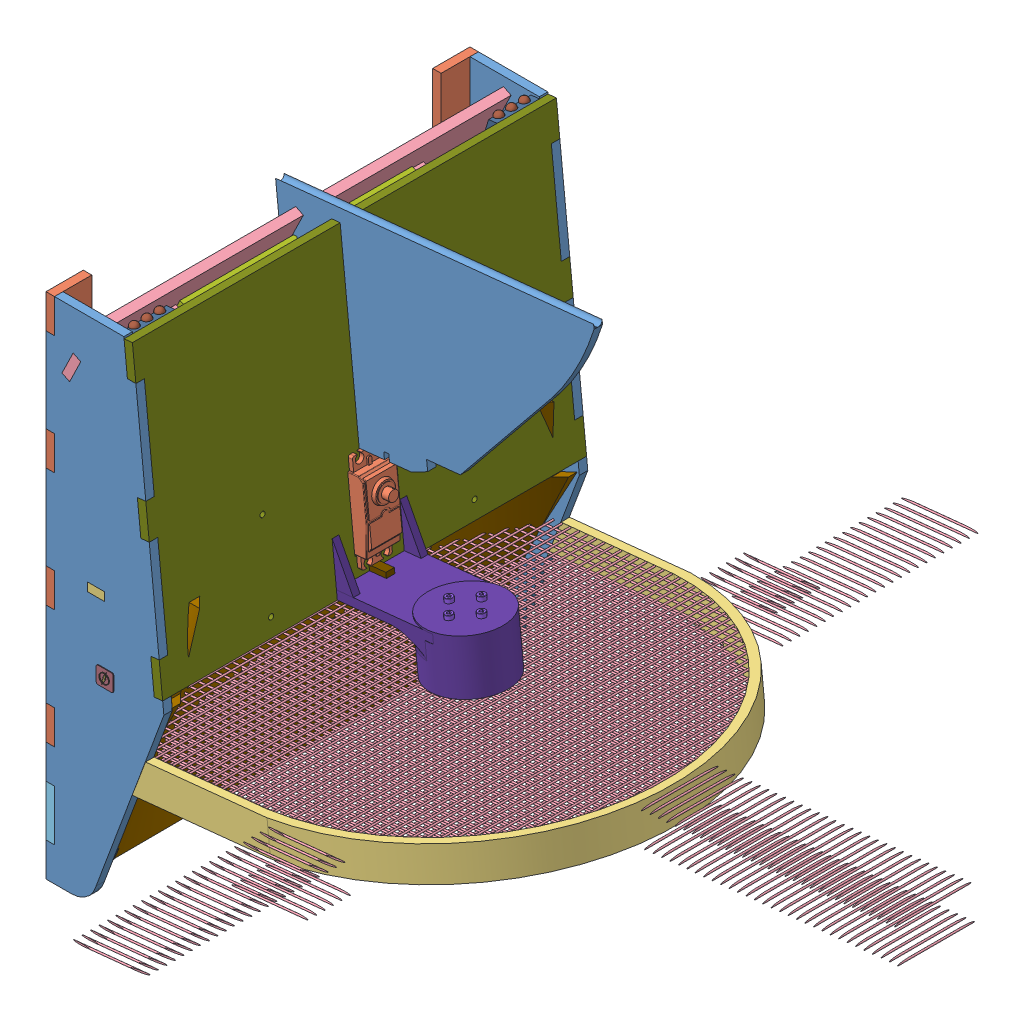
SolidWorks assembly AssStructSimu, configuration Défaut. Lengths in mm.
Overall size (253.25 324.59 251.6).
1750 component instances, 226 part files, 11 mates.
Components (placement in the parent):
- AssBase-1: AssBase [Défaut] at (36.5482 -71.0398 34.0612) size (86.08 302.3 251.6)
  - AssD-1: AssD [Défaut] at (39.0992 31.0201 8.5) size (69.5 300 22)
    - P1-1: P1 [Défaut] at (-95.5819 194.6656 377.5) size (69.5 300 5)
    - P5-1: P5 [Défaut] at (-100.5819 -35.3344 360.5) x (0 1 0) z (1 0 0) size (230 22 5)
  - AssG-1: AssG [Défaut] at (39.0992 31.0201 -236.5) size (69.5 300 22)
    - P1-1: P1 [Défaut] at (-95.5819 194.6656 377.5) size (69.5 300 5)
    - P5-1: P5 [Défaut] at (-95.5819 -35.3344 399.5) x (0 1 0) z (-1 0 0) size (230 22 5)
  - P7-1: P7 [Défaut] at (-1.4828 89.6857 370.5) x (0 0 -1) z (0 -1 0) size (250 54.5 5)
  - P4-1: P4 [Défaut] at (-63.2363 165.9323 386) x (0 0 -1) z (0.898794 -0.438371 0) size (250 60.5 66.27)
  - P3-1: P3 [Défaut] at (-56.4828 -74.3143 146) x (0 0 1) z (-1 0 0) size (250 70 5)
  - P4b-1: P4b [Défaut] at (-58.7423 163.7404 190) x (0 0 1) z (0.438371 0.898794 0) size (152 56 2)
  - battery-1: battery [Défaut] at (-39.0156 204.1861 197.5) x (0 0 1) z (0.898794 -0.438371 0) size (137 43 30)
  - socket head cap screw 4762_din-1: socket head cap screw 4762_din [EN ISO 4762 M3 x 10 - 10N] at (-27.7008 145.2627 193) x (0.438371 0.898794 0) z (0 0 -1) size (13 5.5 5.5)
  - socket head cap screw 4762_din-2: socket head cap screw 4762_din [EN ISO 4762 M3 x 10 - 10N] at (-27.7008 145.2627 339) x (0.438371 0.898794 0) z (-0.791285 0.385936 -0.474259) size (13 5.5 5.5)
  - socket head cap screw 4762_din-3: socket head cap screw 4762_din [EN ISO 4762 M3 x 10 - 10N] at (-42.0815 152.2766 339) x (0.438371 0.898794 0) z (-0.001489 0.000726 -0.999999) size (13 5.5 5.5)
  - socket head cap screw 4762_din-4: socket head cap screw 4762_din [EN ISO 4762 M3 x 10 - 10N] at (-42.0815 152.2766 193) x (0.438371 0.898794 0) z (-0.031331 0.015281 -0.999392) size (13 5.5 5.5)
  - P11-1: P11 [Défaut] at (-57.5734 -73.9703 146.7843) x (0.005072 0 0.999987) z (0.006197 0.999981 -0.000031) size (240 65 164)
  - AssPhare-1: AssPhare [Défaut] at (-52.8518 -67.6977 411) x (0 1 0) z (0 0 -1) size (40.8 8 27.06)
    - piece_led-1: piece_led [Défaut] at (-6.6166 -3.631 25) size (7 8 25)
    - LED 5mm-1: LED 5mm [Valor predeterminado] at (-0.1166 0.369 30) x (0 0 1) z (-1 0 0) size (5.5 6 35.8)
    - LED 5mm-2: LED 5mm [Valor predeterminado] at (-0.1166 0.369 37.5) x (0 0 1) z (-1 0 0) size (5.5 6 35.8)
    - LED 5mm-3: LED 5mm [Valor predeterminado] at (-0.1166 0.369 45) x (0 0 1) z (-1 0 0) size (5.5 6 35.8)
  - AssPhare-2: AssPhare [Défaut] at (-52.8518 -67.6977 196) x (0 1 0) z (0 0 -1) size (40.8 8 27.06)
    - piece_led-1: piece_led [Défaut] at (-6.6166 -3.631 25) size (7 8 25)
    - LED 5mm-1: LED 5mm [Valor predeterminado] at (-0.1166 0.369 30) x (0 0 1) z (-1 0 0) size (5.5 6 35.8)
    - LED 5mm-2: LED 5mm [Valor predeterminado] at (-0.1166 0.369 37.5) x (0 0 1) z (-1 0 0) size (5.5 6 35.8)
    - LED 5mm-3: LED 5mm [Valor predeterminado] at (-0.1166 0.369 45) x (0 0 1) z (-1 0 0) size (5.5 6 35.8)
  - AssLogo-1: AssLogo [Défaut] at (-27.8835 45.1673 148.1054) x (-1 0 0) z (0 0 -1) size (10 10 0.8)
    - logo1-1: logo1 [Défaut] at (-6.5271 -4.4734 6.5054) size (5.8 7.71 0.4)
    - logo2-1: logo2 [Défaut] at (-6.4007 -4.4815 7.1054) size (10 10 0.4)
  - AssLogo-2: AssLogo [Défaut] at (-25.082 45.1673 383.8946) size (10 10 0.8)
    - logo1-1: logo1 [Défaut] at (-6.5271 -4.4734 6.5054) size (5.8 7.71 0.4)
    - logo2-1: logo2 [Défaut] at (-6.4007 -4.4815 7.1054) size (10 10 0.4)
  - support2-1: support2 [Défaut] at (-61.5648 191.7124 276) x (-0.017452 -0.999848 0) z (0.999848 -0.017452 0) size (75 20 10)
  - socket head cap screw 4762_din-5: socket head cap screw 4762_din [EN ISO 4762 M3 x 5 - 5N] at (-61.652 186.7132 269.3333) x (0.999848 -0.017452 0) z (-0.002158 -0.123615 0.992328) size (8 5.5 5.5)
  - socket head cap screw 4762_din-6: socket head cap screw 4762_din [EN ISO 4762 M3 x 5 - 5N] at (-61.652 186.7132 262.6667) x (0.999848 -0.017452 0) z (0 0 1) size (8 5.5 5.5)
  - socket head cap screw 4762_din-7: socket head cap screw 4762_din [EN ISO 4762 M3 x 25 - 18N] at (-55.2963 121.0922 253) x (0 0 1) z (-1 0 0) size (28 5.5 5.5)
  - hex nut style 1 gradeab_din-1: hex nut style 1 gradeab_din [Hexagon Nut ISO 4032 - M3 - W - N] at (-55.2963 121.0922 276) x (-0.923728 -0.383049 0) z (0 0 -1) size (5.5 6.35 2.4)
- AssToitMot-1: AssToitMot [Défaut] at (-168.5238 43.6961 238.494) x (0 0 -1) z (0.9948 0.101852 0) size (250 207.5 205)
  - AssToit-1: AssToit [Défaut] at (-23.0702 -16.5789 -3.7148) size (250 207.5 205)
    - P8-1: P8 [Défaut] at (-38.4971 122.5921 203.5) size (250 175 5)
    - P12-1: P12 [Défaut] at (-60.4971 -63.4079 265.5) x (1 0 0) z (0 -1 0) size (44.28 76.64 55)
    - P13-1: P13 [Défaut] at (-35.9971 -52.8579 208.5) x (0 0 1) z (-1 0 0) size (64 15.55 5)
    - P10_2-1: P10_2 [Défaut] at (-35.9971 111.5921 171) x (0 0 1) z (-1 0 0) size (188.5 117.6 5)
  - Parallax-Servo_DUMMY-1: Parallax-Servo_DUMMY [Défaut] at (-61.6002 -51.5207 216.6662) x (1 0 0) z (0 1 0) size (20.07 42.67 55.64)
  - socket head cap screw 4762_din-1: socket head cap screw 4762_din [EN ISO 4762 M2.5 x 5 - 5N] at (-51.9272 -76.4868 259.2852) x (0 -1 0) z (-0.546944 0 0.837169) size (7.5 4.5 4.5)
  - socket head cap screw 4762_din-2: socket head cap screw 4762_din [EN ISO 4762 M2.5 x 5 - 5N] at (-61.5672 -76.4868 268.9252) x (0 -1 0) z (-0.546944 0 0.837169) size (7.5 4.5 4.5)
  - socket head cap screw 4762_din-3: socket head cap screw 4762_din [EN ISO 4762 M2.5 x 5 - 5N] at (-71.2072 -76.4868 259.2852) x (0 -1 0) z (-0.546944 0 0.837169) size (7.5 4.5 4.5)
  - socket head cap screw 4762_din-4: socket head cap screw 4762_din [EN ISO 4762 M2.5 x 5 - 5N] at (-61.5672 -76.4868 249.6452) x (0 -1 0) z (-0.546944 0 0.837169) size (7.5 4.5 4.5)
  - AssPhare-1: AssPhare [Défaut] at (8.4328 83.3966 196.1542) x (0 -1 0) z (1 0 0) size (40.8 8 27.06)
    - piece_led-1: piece_led [Défaut] at (-6.6166 -3.631 25) size (7 8 25)
    - LED 5mm-1: LED 5mm [Valor predeterminado] at (-0.1166 0.369 30) x (0 0 1) z (-1 0 0) size (5.5 6 35.8)
    - LED 5mm-2: LED 5mm [Valor predeterminado] at (-0.1166 0.369 37.5) x (0 0 1) z (-1 0 0) size (5.5 6 35.8)
    - LED 5mm-3: LED 5mm [Valor predeterminado] at (-0.1166 0.369 45) x (0 0 1) z (-1 0 0) size (5.5 6 35.8)
  - AssPhare-2: AssPhare [Défaut] at (-206.5672 83.3966 196.1542) x (0 -1 0) z (1 0 0) size (40.8 8 27.06)
    - piece_led-1: piece_led [Défaut] at (-6.6166 -3.631 25) size (7 8 25)
    - LED 5mm-1: LED 5mm [Valor predeterminado] at (-0.1166 0.369 30) x (0 0 1) z (-1 0 0) size (5.5 6 35.8)
    - LED 5mm-2: LED 5mm [Valor predeterminado] at (-0.1166 0.369 37.5) x (0 0 1) z (-1 0 0) size (5.5 6 35.8)
    - LED 5mm-3: LED 5mm [Valor predeterminado] at (-0.1166 0.369 45) x (0 0 1) z (-1 0 0) size (5.5 6 35.8)
- AssProtec-1: AssProtec [Défaut] at (86.6746 190.4649 284.6351) x (0 0 -1) z (0.101852 -0.9948 0) size (250 237.46 20)
  - protec3c-1: protec3c [Défaut] at (-140.4261 -87.7568 240) size (250 197 20)
  - AssGrillage-1: AssGrillage [Défaut] at (-370.4609 -132.5428 258.3161) x (0 0 -1) z (1 0 0) size (2.02 237.05 250)
    - barreau-1: barreau [Défaut] at (-1.1839 0.254 200) size (1 1 400)
    - barreau-3: barreau [Défaut] at (-1.1839 5.254 200) size (1 1 400)
    - barreau-4: barreau [Défaut] at (-1.1839 10.254 200) size (1 1 400)
    - barreau-5: barreau [Défaut] at (-1.1839 15.254 200) size (1 1 400)
    - barreau-6: barreau [Défaut] at (-1.1839 20.254 200) size (1 1 400)
    - barreau-7: barreau [Défaut] at (-1.1839 25.254 200) size (1 1 400)
    - barreau-8: barreau [Défaut] at (-1.1839 30.254 200) size (1 1 400)
    - barreau-9: barreau [Défaut] at (-1.1839 35.254 200) size (1 1 400)
    - barreau-10: barreau [Défaut] at (-1.1839 40.254 200) size (1 1 400)
    - barreau-11: barreau [Défaut] at (-1.1839 45.254 200) size (1 1 400)
    - barreau-12: barreau [Défaut] at (-1.1839 50.254 200) size (1 1 400)
    - barreau-13: barreau [Défaut] at (-1.1839 55.254 200) size (1 1 400)
    - barreau-14: barreau [Défaut] at (-1.1839 60.254 200) size (1 1 400)
    - barreau-15: barreau [Défaut] at (-1.1839 65.254 200) size (1 1 400)
    - barreau-16: barreau [Défaut] at (-1.1839 70.254 200) size (1 1 400)
    - barreau-17: barreau [Défaut] at (-1.1839 75.254 200) size (1 1 400)
    - barreau-18: barreau [Défaut] at (-1.1839 80.254 200) size (1 1 400)
    - barreau-19: barreau [Défaut] at (-1.1839 85.254 200) size (1 1 400)
    - barreau-20: barreau [Défaut] at (-1.1839 90.254 200) size (1 1 400)
    - barreau-21: barreau [Défaut] at (-1.1839 95.254 200) size (1 1 400)
    - barreau-22: barreau [Défaut] at (-1.1839 100.254 200) size (1 1 400)
    - barreau-23: barreau [Défaut] at (-1.1839 105.254 200) size (1 1 400)
    - barreau-24: barreau [Défaut] at (-1.1839 110.254 200) size (1 1 400)
    - barreau-25: barreau [Défaut] at (-1.1839 115.254 200) size (1 1 400)
    - barreau-26: barreau [Défaut] at (-1.1839 120.254 200) size (1 1 400)
    - barreau-27: barreau [Défaut] at (-1.1839 125.254 200) size (1 1 400)
    - barreau-28: barreau [Défaut] at (-1.1839 130.254 200) size (1 1 400)
    - barreau-29: barreau [Défaut] at (-1.1839 135.254 200) size (1 1 400)
    - barreau-30: barreau [Défaut] at (-1.1839 140.254 200) size (1 1 400)
    - barreau-31: barreau [Défaut] at (-1.1839 145.254 200) size (1 1 400)
    - barreau-32: barreau [Défaut] at (-1.1839 150.254 200) size (1 1 400)
    - barreau-33: barreau [Défaut] at (-1.1839 155.254 200) size (1 1 400)
    - barreau-34: barreau [Défaut] at (-1.1839 160.254 200) size (1 1 400)
    - barreau-35: barreau [Défaut] at (-1.1839 165.254 200) size (1 1 400)
    - barreau-36: barreau [Défaut] at (-1.1839 170.254 200) size (1 1 400)
    - barreau-37: barreau [Défaut] at (-1.1839 175.254 200) size (1 1 400)
    - barreau-38: barreau [Défaut] at (-1.1839 180.254 200) size (1 1 400)
    - barreau-39: barreau [Défaut] at (-1.1839 185.254 200) size (1 1 400)
    - barreau-40: barreau [Défaut] at (-1.1839 190.254 200) size (1 1 400)
    - barreau-41: barreau [Défaut] at (-1.1839 195.254 200) size (1 1 400)
    - barreau-42: barreau [Défaut] at (-0.1839 -1.5314 598.7823) x (0.998922 0 0.04641) z (0 1 0) size (1 1 400)
    - barreau-43: barreau [Défaut] at (-1.1839 200.254 200) size (1 1 400)
    - barreau-44: barreau [Défaut] at (-1.1839 205.254 200) size (1 1 400)
    - barreau-45: barreau [Défaut] at (-1.1839 210.254 200) size (1 1 400)
    - barreau-46: barreau [Défaut] at (-1.1839 215.254 200) size (1 1 400)
    - barreau-47: barreau [Défaut] at (-1.1839 220.254 200) size (1 1 400)
    - barreau-48: barreau [Défaut] at (-1.1839 225.254 200) size (1 1 400)
    - barreau-49: barreau [Défaut] at (-1.1839 230.254 200) size (1 1 400)
    - barreau-50: barreau [Défaut] at (-1.1839 235.254 200) size (1 1 400)
    - barreau-51: barreau [Défaut] at (-1.1839 240.254 200) size (1 1 400)
    - barreau-52: barreau [Défaut] at (-1.1839 245.254 200) size (1 1 400)
    - barreau-53: barreau [Défaut] at (-1.1839 250.254 200) size (1 1 400)
    - barreau-54: barreau [Défaut] at (-1.1839 255.254 200) size (1 1 400)
    - barreau-55: barreau [Défaut] at (-1.1839 260.254 200) size (1 1 400)
    - barreau-56: barreau [Défaut] at (-1.1839 265.254 200) size (1 1 400)
    - barreau-57: barreau [Défaut] at (-1.1839 270.254 200) size (1 1 400)
    - barreau-58: barreau [Défaut] at (-1.1839 275.254 200) size (1 1 400)
    - barreau-59: barreau [Défaut] at (-1.1839 280.254 200) size (1 1 400)
    - barreau-60: barreau [Défaut] at (-1.1839 285.254 200) size (1 1 400)
    - barreau-61: barreau [Défaut] at (-1.1839 290.254 200) size (1 1 400)
    - barreau-62: barreau [Défaut] at (-1.1839 295.254 200) size (1 1 400)
    - barreau-63: barreau [Défaut] at (-1.1839 300.254 200) size (1 1 400)
    - barreau-64: barreau [Défaut] at (-1.1839 305.254 200) size (1 1 400)
    - barreau-65: barreau [Défaut] at (-1.1839 310.254 200) size (1 1 400)
    - barreau-66: barreau [Défaut] at (-1.1839 315.254 200) size (1 1 400)
    - barreau-67: barreau [Défaut] at (-1.1839 320.254 200) size (1 1 400)
    - barreau-68: barreau [Défaut] at (-1.1839 325.254 200) size (1 1 400)
    - barreau-69: barreau [Défaut] at (-1.1839 330.254 200) size (1 1 400)
    - barreau-70: barreau [Défaut] at (-1.1839 335.254 200) size (1 1 400)
    - barreau-71: barreau [Défaut] at (-1.1839 340.254 200) size (1 1 400)
    - barreau-72: barreau [Défaut] at (-1.1839 345.254 200) size (1 1 400)
    - barreau-73: barreau [Défaut] at (-1.1839 350.254 200) size (1 1 400)
    - barreau-74: barreau [Défaut] at (-1.1839 355.254 200) size (1 1 400)
    - barreau-75: barreau [Défaut] at (-1.1839 360.254 200) size (1 1 400)
    - barreau-76: barreau [Défaut] at (-1.1839 365.254 200) size (1 1 400)
    - barreau-77: barreau [Défaut] at (-1.1839 370.254 200) size (1 1 400)
    - barreau-78: barreau [Défaut] at (-1.1839 375.254 200) size (1 1 400)
    - barreau-79: barreau [Défaut] at (-1.1839 380.254 200) size (1 1 400)
    - barreau-80: barreau [Défaut] at (-1.1839 385.254 200) size (1 1 400)
    - barreau-81: barreau [Défaut] at (-1.1839 390.254 200) size (1 1 400)
    - barreau-82: barreau [Défaut] at (-1.1839 395.254 200) size (1 1 400)
    - barreau-136: barreau [Défaut] at (-0.1839 -1.5314 593.7823) x (0.998922 0 0.04641) z (0 1 0) size (1 1 400)
    - barreau-137: barreau [Défaut] at (-0.1839 -1.5314 588.7823) x (0.998922 0 0.04641) z (0 1 0) size (1 1 400)
    - barreau-138: barreau [Défaut] at (-0.1839 -1.5314 583.7823) x (0.998922 0 0.04641) z (0 1 0) size (1 1 400)
    - barreau-139: barreau [Défaut] at (-0.1839 -1.5314 578.7823) x (0.998922 0 0.04641) z (0 1 0) size (1 1 400)
    - barreau-140: barreau [Défaut] at (-0.1839 -1.5314 573.7823) x (0.998922 0 0.04641) z (0 1 0) size (1 1 400)
    - barreau-141: barreau [Défaut] at (-0.1839 -1.5314 568.7823) x (0.998922 0 0.04641) z (0 1 0) size (1 1 400)
    - barreau-142: barreau [Défaut] at (-0.1839 -1.5314 563.7823) x (0.998922 0 0.04641) z (0 1 0) size (1 1 400)
    - barreau-143: barreau [Défaut] at (-0.1839 -1.5314 558.7823) x (0.998922 0 0.04641) z (0 1 0) size (1 1 400)
    - barreau-144: barreau [Défaut] at (-0.1839 -1.5314 553.7823) x (0.998922 0 0.04641) z (0 1 0) size (1 1 400)
    - barreau-145: barreau [Défaut] at (-0.1839 -1.5314 548.7823) x (0.998922 0 0.04641) z (0 1 0) size (1 1 400)
    - barreau-146: barreau [Défaut] at (-0.1839 -1.5314 543.7823) x (0.998922 0 0.04641) z (0 1 0) size (1 1 400)
    - barreau-147: barreau [Défaut] at (-0.1839 -1.5314 538.7823) x (0.998922 0 0.04641) z (0 1 0) size (1 1 400)
    - barreau-148: barreau [Défaut] at (-0.1839 -1.5314 533.7823) x (0.998922 0 0.04641) z (0 1 0) size (1 1 400)
    - barreau-149: barreau [Défaut] at (-0.1839 -1.5314 528.7823) x (0.998922 0 0.04641) z (0 1 0) size (1 1 400)
    - barreau-150: barreau [Défaut] at (-0.1839 -1.5314 523.7823) x (0.998922 0 0.04641) z (0 1 0) size (1 1 400)
    - barreau-151: barreau [Défaut] at (-0.1839 -1.5314 518.7823) x (0.998922 0 0.04641) z (0 1 0) size (1 1 400)
    - barreau-152: barreau [Défaut] at (-0.1839 -1.5314 513.7823) x (0.998922 0 0.04641) z (0 1 0) size (1 1 400)
    - barreau-153: barreau [Défaut] at (-0.1839 -1.5314 508.7823) x (0.998922 0 0.04641) z (0 1 0) size (1 1 400)
    - barreau-154: barreau [Défaut] at (-0.1839 -1.5314 503.7823) x (0.998922 0 0.04641) z (0 1 0) size (1 1 400)
    - barreau-155: barreau [Défaut] at (-0.1839 -1.5314 498.7823) x (0.998922 0 0.04641) z (0 1 0) size (1 1 400)
    - barreau-156: barreau [Défaut] at (-0.1839 -1.5314 493.7823) x (0.998922 0 0.04641) z (0 1 0) size (1 1 400)
    - barreau-157: barreau [Défaut] at (-0.1839 -1.5314 488.7823) x (0.998922 0 0.04641) z (0 1 0) size (1 1 400)
    - barreau-158: barreau [Défaut] at (-0.1839 -1.5314 483.7823) x (0.998922 0 0.04641) z (0 1 0) size (1 1 400)
    - barreau-159: barreau [Défaut] at (-0.1839 -1.5314 478.7823) x (0.998922 0 0.04641) z (0 1 0) size (1 1 400)
    - barreau-160: barreau [Défaut] at (-0.1839 -1.5314 473.7823) x (0.998922 0 0.04641) z (0 1 0) size (1 1 400)
    - barreau-161: barreau [Défaut] at (-0.1839 -1.5314 468.7823) x (0.998922 0 0.04641) z (0 1 0) size (1 1 400)
    - barreau-162: barreau [Défaut] at (-0.1839 -1.5314 463.7823) x (0.998922 0 0.04641) z (0 1 0) size (1 1 400)
    - barreau-163: barreau [Défaut] at (-0.1839 -1.5314 458.7823) x (0.998922 0 0.04641) z (0 1 0) size (1 1 400)
    - barreau-164: barreau [Défaut] at (-0.1839 -1.5314 453.7823) x (0.998922 0 0.04641) z (0 1 0) size (1 1 400)
    - barreau-165: barreau [Défaut] at (-0.1839 -1.5314 448.7823) x (0.998922 0 0.04641) z (0 1 0) size (1 1 400)
    - barreau-166: barreau [Défaut] at (-0.1839 -1.5314 443.7823) x (0.998922 0 0.04641) z (0 1 0) size (1 1 400)
    - barreau-167: barreau [Défaut] at (-0.1839 -1.5314 438.7823) x (0.998922 0 0.04641) z (0 1 0) size (1 1 400)
    - barreau-168: barreau [Défaut] at (-0.1839 -1.5314 433.7823) x (0.998922 0 0.04641) z (0 1 0) size (1 1 400)
    - barreau-169: barreau [Défaut] at (-0.1839 -1.5314 428.7823) x (0.998922 0 0.04641) z (0 1 0) size (1 1 400)
    - barreau-170: barreau [Défaut] at (-0.1839 -1.5314 423.7823) x (0.998922 0 0.04641) z (0 1 0) size (1 1 400)
    - barreau-171: barreau [Défaut] at (-0.1839 -1.5314 418.7823) x (0.998922 0 0.04641) z (0 1 0) size (1 1 400)
    - barreau-172: barreau [Défaut] at (-0.1839 -1.5314 413.7823) x (0.998922 0 0.04641) z (0 1 0) size (1 1 400)
    - barreau-173: barreau [Défaut] at (-0.1839 -1.5314 408.7823) x (0.998922 0 0.04641) z (0 1 0) size (1 1 400)
    - barreau-174: barreau [Défaut] at (-0.1839 -1.5314 403.7823) x (0.998922 0 0.04641) z (0 1 0) size (1 1 400)
    - barreau-175: barreau [Défaut] at (-0.1839 -1.5314 398.7823) x (0.998922 0 0.04641) z (0 1 0) size (1 1 400)
    - barreau-176: barreau [Défaut] at (-0.1839 -1.5314 393.7823) x (0.998922 0 0.04641) z (0 1 0) size (1 1 400)
    - barreau-177: barreau [Défaut] at (-0.1839 -1.5314 388.7823) x (0.998922 0 0.04641) z (0 1 0) size (1 1 400)
    - barreau-178: barreau [Défaut] at (-0.1839 -1.5314 383.7823) x (0.998922 0 0.04641) z (0 1 0) size (1 1 400)
    - barreau-179: barreau [Défaut] at (-0.1839 -1.5314 378.7823) x (0.998922 0 0.04641) z (0 1 0) size (1 1 400)
    - barreau-180: barreau [Défaut] at (-0.1839 -1.5314 373.7823) x (0.998922 0 0.04641) z (0 1 0) size (1 1 400)
    - barreau-181: barreau [Défaut] at (-0.1839 -1.5314 368.7823) x (0.998922 0 0.04641) z (0 1 0) size (1 1 400)
    - barreau-182: barreau [Défaut] at (-0.1839 -1.5314 363.7823) x (0.998922 0 0.04641) z (0 1 0) size (1 1 400)
    - barreau-183: barreau [Défaut] at (-0.1839 -1.5314 358.7823) x (0.998922 0 0.04641) z (0 1 0) size (1 1 400)
    - barreau-184: barreau [Défaut] at (-0.1839 -1.5314 353.7823) x (0.998922 0 0.04641) z (0 1 0) size (1 1 400)
    - barreau-185: barreau [Défaut] at (-0.1839 -1.5314 348.7823) x (0.998922 0 0.04641) z (0 1 0) size (1 1 400)
    - barreau-186: barreau [Défaut] at (-0.1839 -1.5314 343.7823) x (0.998922 0 0.04641) z (0 1 0) size (1 1 400)
    - barreau-187: barreau [Défaut] at (-0.1839 -1.5314 338.7823) x (0.998922 0 0.04641) z (0 1 0) size (1 1 400)
    - barreau-188: barreau [Défaut] at (-0.1839 -1.5314 333.7823) x (0.998922 0 0.04641) z (0 1 0) size (1 1 400)
    - barreau-189: barreau [Défaut] at (-0.1839 -1.5314 328.7823) x (0.998922 0 0.04641) z (0 1 0) size (1 1 400)
    - barreau-190: barreau [Défaut] at (-0.1839 -1.5314 323.7823) x (0.998922 0 0.04641) z (0 1 0) size (1 1 400)
    - barreau-191: barreau [Défaut] at (-0.1839 -1.5314 318.7823) x (0.998922 0 0.04641) z (0 1 0) size (1 1 400)
    - barreau-192: barreau [Défaut] at (-0.1839 -1.5314 313.7823) x (0.998922 0 0.04641) z (0 1 0) size (1 1 400)
    - barreau-193: barreau [Défaut] at (-0.1839 -1.5314 308.7823) x (0.998922 0 0.04641) z (0 1 0) size (1 1 400)
    - barreau-194: barreau [Défaut] at (-0.1839 -1.5314 303.7823) x (0.998922 0 0.04641) z (0 1 0) size (1 1 400)
    - barreau-195: barreau [Défaut] at (-0.1839 -1.5314 298.7823) x (0.998922 0 0.04641) z (0 1 0) size (1 1 400)
    - barreau-196: barreau [Défaut] at (-0.1839 -1.5314 293.7823) x (0.998922 0 0.04641) z (0 1 0) size (1 1 400)
    - barreau-197: barreau [Défaut] at (-0.1839 -1.5314 288.7823) x (0.998922 0 0.04641) z (0 1 0) size (1 1 400)
    - barreau-198: barreau [Défaut] at (-0.1839 -1.5314 283.7823) x (0.998922 0 0.04641) z (0 1 0) size (1 1 400)
    - barreau-199: barreau [Défaut] at (-0.1839 -1.5314 278.7823) x (0.998922 0 0.04641) z (0 1 0) size (1 1 400)
    - barreau-200: barreau [Défaut] at (-0.1839 -1.5314 273.7823) x (0.998922 0 0.04641) z (0 1 0) size (1 1 400)
    - barreau-201: barreau [Défaut] at (-0.1839 -1.5314 268.7823) x (0.998922 0 0.04641) z (0 1 0) size (1 1 400)
    - barreau-202: barreau [Défaut] at (-0.1839 -1.5314 263.7823) x (0.998922 0 0.04641) z (0 1 0) size (1 1 400)
    - barreau-203: barreau [Défaut] at (-0.1839 -1.5314 258.7823) x (0.998922 0 0.04641) z (0 1 0) size (1 1 400)
    - barreau-204: barreau [Défaut] at (-0.1839 -1.5314 253.7823) x (0.998922 0 0.04641) z (0 1 0) size (1 1 400)
    - barreau-205: barreau [Défaut] at (-0.1839 -1.5314 248.7823) x (0.998922 0 0.04641) z (0 1 0) size (1 1 400)
    - barreau-206: barreau [Défaut] at (-0.1839 -1.5314 243.7823) x (0.998922 0 0.04641) z (0 1 0) size (1 1 400)
    - barreau-207: barreau [Défaut] at (-0.1839 -1.5314 238.7823) x (0.998922 0 0.04641) z (0 1 0) size (1 1 400)
    - barreau-208: barreau [Défaut] at (-0.1839 -1.5314 233.7823) x (0.998922 0 0.04641) z (0 1 0) size (1 1 400)
    - barreau-209: barreau [Défaut] at (-0.1839 -1.5314 228.7823) x (0.998922 0 0.04641) z (0 1 0) size (1 1 400)
    - barreau-210: barreau [Défaut] at (-0.1839 -1.5314 223.7823) x (0.998922 0 0.04641) z (0 1 0) size (1 1 400)
    - barreau-211: barreau [Défaut] at (-0.1839 -1.5314 218.7823) x (0.998922 0 0.04641) z (0 1 0) size (1 1 400)
    - barreau-212: barreau [Défaut] at (-0.1839 -1.5314 213.7823) x (0.998922 0 0.04641) z (0 1 0) size (1 1 400)
    - barreau-213: barreau [Défaut] at (-0.1839 -1.5314 208.7823) x (0.998922 0 0.04641) z (0 1 0) size (1 1 400)
    - barreau-214: barreau [Défaut] at (-0.1839 -1.5314 203.7823) x (0.998922 0 0.04641) z (0 1 0) size (1 1 400)
  - AssGrillage-2: AssGrillage [Défaut] at (339.6086 -132.5428 241.6839) x (0 0 1) z (-1 0 0) size (2.02 237.05 250)
    - barreau-1: barreau [Défaut] at (-1.1839 0.254 200) size (1 1 400)
    - barreau-3: barreau [Défaut] at (-1.1839 5.254 200) size (1 1 400)
    - barreau-4: barreau [Défaut] at (-1.1839 10.254 200) size (1 1 400)
    - barreau-5: barreau [Défaut] at (-1.1839 15.254 200) size (1 1 400)
    - barreau-6: barreau [Défaut] at (-1.1839 20.254 200) size (1 1 400)
    - barreau-7: barreau [Défaut] at (-1.1839 25.254 200) size (1 1 400)
    - barreau-8: barreau [Défaut] at (-1.1839 30.254 200) size (1 1 400)
    - barreau-9: barreau [Défaut] at (-1.1839 35.254 200) size (1 1 400)
    - barreau-10: barreau [Défaut] at (-1.1839 40.254 200) size (1 1 400)
    - barreau-11: barreau [Défaut] at (-1.1839 45.254 200) size (1 1 400)
    - barreau-12: barreau [Défaut] at (-1.1839 50.254 200) size (1 1 400)
    - barreau-13: barreau [Défaut] at (-1.1839 55.254 200) size (1 1 400)
    - barreau-14: barreau [Défaut] at (-1.1839 60.254 200) size (1 1 400)
    - barreau-15: barreau [Défaut] at (-1.1839 65.254 200) size (1 1 400)
    - barreau-16: barreau [Défaut] at (-1.1839 70.254 200) size (1 1 400)
    - barreau-17: barreau [Défaut] at (-1.1839 75.254 200) size (1 1 400)
    - barreau-18: barreau [Défaut] at (-1.1839 80.254 200) size (1 1 400)
    - barreau-19: barreau [Défaut] at (-1.1839 85.254 200) size (1 1 400)
    - barreau-20: barreau [Défaut] at (-1.1839 90.254 200) size (1 1 400)
    - barreau-21: barreau [Défaut] at (-1.1839 95.254 200) size (1 1 400)
    - barreau-22: barreau [Défaut] at (-1.1839 100.254 200) size (1 1 400)
    - barreau-23: barreau [Défaut] at (-1.1839 105.254 200) size (1 1 400)
    - barreau-24: barreau [Défaut] at (-1.1839 110.254 200) size (1 1 400)
    - barreau-25: barreau [Défaut] at (-1.1839 115.254 200) size (1 1 400)
    - barreau-26: barreau [Défaut] at (-1.1839 120.254 200) size (1 1 400)
    - barreau-27: barreau [Défaut] at (-1.1839 125.254 200) size (1 1 400)
    - barreau-28: barreau [Défaut] at (-1.1839 130.254 200) size (1 1 400)
    - barreau-29: barreau [Défaut] at (-1.1839 135.254 200) size (1 1 400)
    - barreau-30: barreau [Défaut] at (-1.1839 140.254 200) size (1 1 400)
    - barreau-31: barreau [Défaut] at (-1.1839 145.254 200) size (1 1 400)
    - barreau-32: barreau [Défaut] at (-1.1839 150.254 200) size (1 1 400)
    - barreau-33: barreau [Défaut] at (-1.1839 155.254 200) size (1 1 400)
    - barreau-34: barreau [Défaut] at (-1.1839 160.254 200) size (1 1 400)
    - barreau-35: barreau [Défaut] at (-1.1839 165.254 200) size (1 1 400)
    - barreau-36: barreau [Défaut] at (-1.1839 170.254 200) size (1 1 400)
    - barreau-37: barreau [Défaut] at (-1.1839 175.254 200) size (1 1 400)
    - barreau-38: barreau [Défaut] at (-1.1839 180.254 200) size (1 1 400)
    - barreau-39: barreau [Défaut] at (-1.1839 185.254 200) size (1 1 400)
    - barreau-40: barreau [Défaut] at (-1.1839 190.254 200) size (1 1 400)
    - barreau-41: barreau [Défaut] at (-1.1839 195.254 200) size (1 1 400)
    - barreau-42: barreau [Défaut] at (-0.1839 -1.5314 598.7823) x (0.998922 0 0.04641) z (0 1 0) size (1 1 400)
    - barreau-43: barreau [Défaut] at (-1.1839 200.254 200) size (1 1 400)
    - barreau-44: barreau [Défaut] at (-1.1839 205.254 200) size (1 1 400)
    - barreau-45: barreau [Défaut] at (-1.1839 210.254 200) size (1 1 400)
    - barreau-46: barreau [Défaut] at (-1.1839 215.254 200) size (1 1 400)
    - barreau-47: barreau [Défaut] at (-1.1839 220.254 200) size (1 1 400)
    - barreau-48: barreau [Défaut] at (-1.1839 225.254 200) size (1 1 400)
    - barreau-49: barreau [Défaut] at (-1.1839 230.254 200) size (1 1 400)
    - barreau-50: barreau [Défaut] at (-1.1839 235.254 200) size (1 1 400)
    - barreau-51: barreau [Défaut] at (-1.1839 240.254 200) size (1 1 400)
    - barreau-52: barreau [Défaut] at (-1.1839 245.254 200) size (1 1 400)
    - barreau-53: barreau [Défaut] at (-1.1839 250.254 200) size (1 1 400)
    - barreau-54: barreau [Défaut] at (-1.1839 255.254 200) size (1 1 400)
    - barreau-55: barreau [Défaut] at (-1.1839 260.254 200) size (1 1 400)
    - barreau-56: barreau [Défaut] at (-1.1839 265.254 200) size (1 1 400)
    - barreau-57: barreau [Défaut] at (-1.1839 270.254 200) size (1 1 400)
    - barreau-58: barreau [Défaut] at (-1.1839 275.254 200) size (1 1 400)
    - barreau-59: barreau [Défaut] at (-1.1839 280.254 200) size (1 1 400)
    - barreau-60: barreau [Défaut] at (-1.1839 285.254 200) size (1 1 400)
    - barreau-61: barreau [Défaut] at (-1.1839 290.254 200) size (1 1 400)
    - barreau-62: barreau [Défaut] at (-1.1839 295.254 200) size (1 1 400)
    - barreau-63: barreau [Défaut] at (-1.1839 300.254 200) size (1 1 400)
    - barreau-64: barreau [Défaut] at (-1.1839 305.254 200) size (1 1 400)
    - barreau-65: barreau [Défaut] at (-1.1839 310.254 200) size (1 1 400)
    - barreau-66: barreau [Défaut] at (-1.1839 315.254 200) size (1 1 400)
    - barreau-67: barreau [Défaut] at (-1.1839 320.254 200) size (1 1 400)
    - barreau-68: barreau [Défaut] at (-1.1839 325.254 200) size (1 1 400)
    - barreau-69: barreau [Défaut] at (-1.1839 330.254 200) size (1 1 400)
    - barreau-70: barreau [Défaut] at (-1.1839 335.254 200) size (1 1 400)
    - barreau-71: barreau [Défaut] at (-1.1839 340.254 200) size (1 1 400)
    - barreau-72: barreau [Défaut] at (-1.1839 345.254 200) size (1 1 400)
    - barreau-73: barreau [Défaut] at (-1.1839 350.254 200) size (1 1 400)
    - barreau-74: barreau [Défaut] at (-1.1839 355.254 200) size (1 1 400)
    - barreau-75: barreau [Défaut] at (-1.1839 360.254 200) size (1 1 400)
    - barreau-76: barreau [Défaut] at (-1.1839 365.254 200) size (1 1 400)
    - barreau-77: barreau [Défaut] at (-1.1839 370.254 200) size (1 1 400)
    - barreau-78: barreau [Défaut] at (-1.1839 375.254 200) size (1 1 400)
    - barreau-79: barreau [Défaut] at (-1.1839 380.254 200) size (1 1 400)
    - barreau-80: barreau [Défaut] at (-1.1839 385.254 200) size (1 1 400)
    - barreau-81: barreau [Défaut] at (-1.1839 390.254 200) size (1 1 400)
    - barreau-82: barreau [Défaut] at (-1.1839 395.254 200) size (1 1 400)
    - barreau-136: barreau [Défaut] at (-0.1839 -1.5314 593.7823) x (0.998922 0 0.04641) z (0 1 0) size (1 1 400)
    - barreau-137: barreau [Défaut] at (-0.1839 -1.5314 588.7823) x (0.998922 0 0.04641) z (0 1 0) size (1 1 400)
    - barreau-138: barreau [Défaut] at (-0.1839 -1.5314 583.7823) x (0.998922 0 0.04641) z (0 1 0) size (1 1 400)
    - barreau-139: barreau [Défaut] at (-0.1839 -1.5314 578.7823) x (0.998922 0 0.04641) z (0 1 0) size (1 1 400)
    - barreau-140: barreau [Défaut] at (-0.1839 -1.5314 573.7823) x (0.998922 0 0.04641) z (0 1 0) size (1 1 400)
    - barreau-141: barreau [Défaut] at (-0.1839 -1.5314 568.7823) x (0.998922 0 0.04641) z (0 1 0) size (1 1 400)
    - barreau-142: barreau [Défaut] at (-0.1839 -1.5314 563.7823) x (0.998922 0 0.04641) z (0 1 0) size (1 1 400)
    - barreau-143: barreau [Défaut] at (-0.1839 -1.5314 558.7823) x (0.998922 0 0.04641) z (0 1 0) size (1 1 400)
    - barreau-144: barreau [Défaut] at (-0.1839 -1.5314 553.7823) x (0.998922 0 0.04641) z (0 1 0) size (1 1 400)
    - barreau-145: barreau [Défaut] at (-0.1839 -1.5314 548.7823) x (0.998922 0 0.04641) z (0 1 0) size (1 1 400)
    - barreau-146: barreau [Défaut] at (-0.1839 -1.5314 543.7823) x (0.998922 0 0.04641) z (0 1 0) size (1 1 400)
    - barreau-147: barreau [Défaut] at (-0.1839 -1.5314 538.7823) x (0.998922 0 0.04641) z (0 1 0) size (1 1 400)
    - barreau-148: barreau [Défaut] at (-0.1839 -1.5314 533.7823) x (0.998922 0 0.04641) z (0 1 0) size (1 1 400)
    - barreau-149: barreau [Défaut] at (-0.1839 -1.5314 528.7823) x (0.998922 0 0.04641) z (0 1 0) size (1 1 400)
    - barreau-150: barreau [Défaut] at (-0.1839 -1.5314 523.7823) x (0.998922 0 0.04641) z (0 1 0) size (1 1 400)
    - barreau-151: barreau [Défaut] at (-0.1839 -1.5314 518.7823) x (0.998922 0 0.04641) z (0 1 0) size (1 1 400)
    - barreau-152: barreau [Défaut] at (-0.1839 -1.5314 513.7823) x (0.998922 0 0.04641) z (0 1 0) size (1 1 400)
    - barreau-153: barreau [Défaut] at (-0.1839 -1.5314 508.7823) x (0.998922 0 0.04641) z (0 1 0) size (1 1 400)
    - barreau-154: barreau [Défaut] at (-0.1839 -1.5314 503.7823) x (0.998922 0 0.04641) z (0 1 0) size (1 1 400)
    - barreau-155: barreau [Défaut] at (-0.1839 -1.5314 498.7823) x (0.998922 0 0.04641) z (0 1 0) size (1 1 400)
    - barreau-156: barreau [Défaut] at (-0.1839 -1.5314 493.7823) x (0.998922 0 0.04641) z (0 1 0) size (1 1 400)
    - barreau-157: barreau [Défaut] at (-0.1839 -1.5314 488.7823) x (0.998922 0 0.04641) z (0 1 0) size (1 1 400)
    - barreau-158: barreau [Défaut] at (-0.1839 -1.5314 483.7823) x (0.998922 0 0.04641) z (0 1 0) size (1 1 400)
    - barreau-159: barreau [Défaut] at (-0.1839 -1.5314 478.7823) x (0.998922 0 0.04641) z (0 1 0) size (1 1 400)
    - barreau-160: barreau [Défaut] at (-0.1839 -1.5314 473.7823) x (0.998922 0 0.04641) z (0 1 0) size (1 1 400)
    - barreau-161: barreau [Défaut] at (-0.1839 -1.5314 468.7823) x (0.998922 0 0.04641) z (0 1 0) size (1 1 400)
    - barreau-162: barreau [Défaut] at (-0.1839 -1.5314 463.7823) x (0.998922 0 0.04641) z (0 1 0) size (1 1 400)
    - barreau-163: barreau [Défaut] at (-0.1839 -1.5314 458.7823) x (0.998922 0 0.04641) z (0 1 0) size (1 1 400)
    - barreau-164: barreau [Défaut] at (-0.1839 -1.5314 453.7823) x (0.998922 0 0.04641) z (0 1 0) size (1 1 400)
    - barreau-165: barreau [Défaut] at (-0.1839 -1.5314 448.7823) x (0.998922 0 0.04641) z (0 1 0) size (1 1 400)
    - barreau-166: barreau [Défaut] at (-0.1839 -1.5314 443.7823) x (0.998922 0 0.04641) z (0 1 0) size (1 1 400)
    - barreau-167: barreau [Défaut] at (-0.1839 -1.5314 438.7823) x (0.998922 0 0.04641) z (0 1 0) size (1 1 400)
    - barreau-168: barreau [Défaut] at (-0.1839 -1.5314 433.7823) x (0.998922 0 0.04641) z (0 1 0) size (1 1 400)
    - barreau-169: barreau [Défaut] at (-0.1839 -1.5314 428.7823) x (0.998922 0 0.04641) z (0 1 0) size (1 1 400)
    - barreau-170: barreau [Défaut] at (-0.1839 -1.5314 423.7823) x (0.998922 0 0.04641) z (0 1 0) size (1 1 400)
    - barreau-171: barreau [Défaut] at (-0.1839 -1.5314 418.7823) x (0.998922 0 0.04641) z (0 1 0) size (1 1 400)
    - barreau-172: barreau [Défaut] at (-0.1839 -1.5314 413.7823) x (0.998922 0 0.04641) z (0 1 0) size (1 1 400)
    - barreau-173: barreau [Défaut] at (-0.1839 -1.5314 408.7823) x (0.998922 0 0.04641) z (0 1 0) size (1 1 400)
    - barreau-174: barreau [Défaut] at (-0.1839 -1.5314 403.7823) x (0.998922 0 0.04641) z (0 1 0) size (1 1 400)
    - barreau-175: barreau [Défaut] at (-0.1839 -1.5314 398.7823) x (0.998922 0 0.04641) z (0 1 0) size (1 1 400)
    - barreau-176: barreau [Défaut] at (-0.1839 -1.5314 393.7823) x (0.998922 0 0.04641) z (0 1 0) size (1 1 400)
    - barreau-177: barreau [Défaut] at (-0.1839 -1.5314 388.7823) x (0.998922 0 0.04641) z (0 1 0) size (1 1 400)
    - barreau-178: barreau [Défaut] at (-0.1839 -1.5314 383.7823) x (0.998922 0 0.04641) z (0 1 0) size (1 1 400)
    - barreau-179: barreau [Défaut] at (-0.1839 -1.5314 378.7823) x (0.998922 0 0.04641) z (0 1 0) size (1 1 400)
    - barreau-180: barreau [Défaut] at (-0.1839 -1.5314 373.7823) x (0.998922 0 0.04641) z (0 1 0) size (1 1 400)
    - barreau-181: barreau [Défaut] at (-0.1839 -1.5314 368.7823) x (0.998922 0 0.04641) z (0 1 0) size (1 1 400)
    - barreau-182: barreau [Défaut] at (-0.1839 -1.5314 363.7823) x (0.998922 0 0.04641) z (0 1 0) size (1 1 400)
    - barreau-183: barreau [Défaut] at (-0.1839 -1.5314 358.7823) x (0.998922 0 0.04641) z (0 1 0) size (1 1 400)
    - barreau-184: barreau [Défaut] at (-0.1839 -1.5314 353.7823) x (0.998922 0 0.04641) z (0 1 0) size (1 1 400)
    - barreau-185: barreau [Défaut] at (-0.1839 -1.5314 348.7823) x (0.998922 0 0.04641) z (0 1 0) size (1 1 400)
    - barreau-186: barreau [Défaut] at (-0.1839 -1.5314 343.7823) x (0.998922 0 0.04641) z (0 1 0) size (1 1 400)
    - barreau-187: barreau [Défaut] at (-0.1839 -1.5314 338.7823) x (0.998922 0 0.04641) z (0 1 0) size (1 1 400)
    - barreau-188: barreau [Défaut] at (-0.1839 -1.5314 333.7823) x (0.998922 0 0.04641) z (0 1 0) size (1 1 400)
    - barreau-189: barreau [Défaut] at (-0.1839 -1.5314 328.7823) x (0.998922 0 0.04641) z (0 1 0) size (1 1 400)
    - barreau-190: barreau [Défaut] at (-0.1839 -1.5314 323.7823) x (0.998922 0 0.04641) z (0 1 0) size (1 1 400)
    - barreau-191: barreau [Défaut] at (-0.1839 -1.5314 318.7823) x (0.998922 0 0.04641) z (0 1 0) size (1 1 400)
    - barreau-192: barreau [Défaut] at (-0.1839 -1.5314 313.7823) x (0.998922 0 0.04641) z (0 1 0) size (1 1 400)
    - barreau-193: barreau [Défaut] at (-0.1839 -1.5314 308.7823) x (0.998922 0 0.04641) z (0 1 0) size (1 1 400)
    - barreau-194: barreau [Défaut] at (-0.1839 -1.5314 303.7823) x (0.998922 0 0.04641) z (0 1 0) size (1 1 400)
    - barreau-195: barreau [Défaut] at (-0.1839 -1.5314 298.7823) x (0.998922 0 0.04641) z (0 1 0) size (1 1 400)
    - barreau-196: barreau [Défaut] at (-0.1839 -1.5314 293.7823) x (0.998922 0 0.04641) z (0 1 0) size (1 1 400)
    - barreau-197: barreau [Défaut] at (-0.1839 -1.5314 288.7823) x (0.998922 0 0.04641) z (0 1 0) size (1 1 400)
    - barreau-198: barreau [Défaut] at (-0.1839 -1.5314 283.7823) x (0.998922 0 0.04641) z (0 1 0) size (1 1 400)
    - barreau-199: barreau [Défaut] at (-0.1839 -1.5314 278.7823) x (0.998922 0 0.04641) z (0 1 0) size (1 1 400)
    - barreau-200: barreau [Défaut] at (-0.1839 -1.5314 273.7823) x (0.998922 0 0.04641) z (0 1 0) size (1 1 400)
    - barreau-201: barreau [Défaut] at (-0.1839 -1.5314 268.7823) x (0.998922 0 0.04641) z (0 1 0) size (1 1 400)
    - barreau-202: barreau [Défaut] at (-0.1839 -1.5314 263.7823) x (0.998922 0 0.04641) z (0 1 0) size (1 1 400)
    - barreau-203: barreau [Défaut] at (-0.1839 -1.5314 258.7823) x (0.998922 0 0.04641) z (0 1 0) size (1 1 400)
    - barreau-204: barreau [Défaut] at (-0.1839 -1.5314 253.7823) x (0.998922 0 0.04641) z (0 1 0) size (1 1 400)
    - barreau-205: barreau [Défaut] at (-0.1839 -1.5314 248.7823) x (0.998922 0 0.04641) z (0 1 0) size (1 1 400)
    - barreau-206: barreau [Défaut] at (-0.1839 -1.5314 243.7823) x (0.998922 0 0.04641) z (0 1 0) size (1 1 400)
    - barreau-207: barreau [Défaut] at (-0.1839 -1.5314 238.7823) x (0.998922 0 0.04641) z (0 1 0) size (1 1 400)
    - barreau-208: barreau [Défaut] at (-0.1839 -1.5314 233.7823) x (0.998922 0 0.04641) z (0 1 0) size (1 1 400)
    - barreau-209: barreau [Défaut] at (-0.1839 -1.5314 228.7823) x (0.998922 0 0.04641) z (0 1 0) size (1 1 400)
    - barreau-210: barreau [Défaut] at (-0.1839 -1.5314 223.7823) x (0.998922 0 0.04641) z (0 1 0) size (1 1 400)
    - barreau-211: barreau [Défaut] at (-0.1839 -1.5314 218.7823) x (0.998922 0 0.04641) z (0 1 0) size (1 1 400)
    - barreau-212: barreau [Défaut] at (-0.1839 -1.5314 213.7823) x (0.998922 0 0.04641) z (0 1 0) size (1 1 400)
    - barreau-213: barreau [Défaut] at (-0.1839 -1.5314 208.7823) x (0.998922 0 0.04641) z (0 1 0) size (1 1 400)
    - barreau-214: barreau [Défaut] at (-0.1839 -1.5314 203.7823) x (0.998922 0 0.04641) z (0 1 0) size (1 1 400)
- AssCarte-1: AssCarte [Défaut] at (38.0121 147.1029 290.772) x (-0.101852 0.9948 0) z (0.9948 0.101852 0) size (66.52 130.57 98.72) (hidden)
  - carte_onduleur_v3-1: carte_onduleur_v3 [Défaut] at (-131.8199 12.0892 20.7912) size (66.52 130.57 82.34)
    - Layer_1-1: Layer_1 [Défaut] at origin size (60 130 1.61)
    - BTN-1: BTN [Défaut] at (-25.5 7.4 0.803) x (0 -1 0) z (0 0 1) size (6.76 3.64 4.37)
      - Open CASCADE STEP translator 6.8 1.2.1-1: Open CASCADE STEP translator 6.8 1.2.1 [Défaut] at origin size (6.76 3.64 4.37)
        - Body_1-1: Body_1 [Défaut] at (-0.5 -2 0) size (6.76 3.64 4.37)
          - =_[0_1_1_3]-1: =_[0_1_1_3] [Défaut] at origin size (6 3.64 4.37)
          - =_[0_1_1_4]-1: =_[0_1_1_4] [Défaut] at origin size (0.38 1 0.67)
          - =_[0_1_1_5]-1: =_[0_1_1_5] [Défaut] at origin size (0.38 1 0.67)
    - CON_IO1-1: CON_IO1 [Défaut] at (-11.3 12.1 0.803) x (0 -1 0) z (0 0 1) size (13 30 57.5)
      - Open CASCADE STEP translator 6.8 1.3.1-1: Open CASCADE STEP translator 6.8 1.3.1 [Défaut] at origin size (13 30 57.5)
        - Body_1_2-1: Body_1_2 [Défaut] at (-3 -15 8) x (0 -1 0) z (-1 0 0) size (30 57.5 13)
          - 1-1: 1 [Défaut] at origin size (30 50 1.61)
          - 10-1: 10 [Défaut] at (-14.395 31.0465 0.803) x (-1 0 0) z (0 0 1) size (5.59 6.35 1.11)
            - =_[0_1_1_4]-1: =_[0_1_1_4] [Défaut] at origin size (5.59 6.35 1.11)
              - 11-1: 11 [Défaut] at (2 3.3 0) x (-1 0 0) z (0 0 1) size (5.59 6.35 1.11)
                - =_[0_1_1_3]_2-1: =_[0_1_1_3]_2 [Défaut] at origin size (0.44 0.55 0.36)
                - =_[0_1_1_4]_2-1: =_[0_1_1_4]_2 [Défaut] at origin size (5.59 4.15 0.36)
                - =_[0_1_1_5]_2-1: =_[0_1_1_5]_2 [Défaut] at origin size (5.35 6.1 1.1)
                - =_[0_1_1_6]-1: =_[0_1_1_6] [Défaut] at origin size (0.44 0.55 0.36)
                - =_[0_1_1_7]-1: =_[0_1_1_7] [Défaut] at origin size (0.44 0.55 0.36)
                - =_[0_1_1_8]-1: =_[0_1_1_8] [Défaut] at origin size (0.44 0.55 0.36)
          - 13-1: 13 [Défaut] at (-12.62 16.6 -0.803) x (-1 0 0) z (0 0 -1) size (5.59 6.35 1.11)
            - =_[0_1_1_13]-1: =_[0_1_1_13] [Défaut] at origin size (5.59 6.35 1.11)
              - 11-1: 11 [Défaut] at (2 3.3 0) x (-1 0 0) z (0 0 1) size (5.59 6.35 1.11)
                - =_[0_1_1_3]_2-1: =_[0_1_1_3]_2 [Défaut] at origin size (0.44 0.55 0.36)
                - =_[0_1_1_4]_2-1: =_[0_1_1_4]_2 [Défaut] at origin size (5.59 4.15 0.36)
                - =_[0_1_1_5]_2-1: =_[0_1_1_5]_2 [Défaut] at origin size (5.35 6.1 1.1)
                - =_[0_1_1_6]-1: =_[0_1_1_6] [Défaut] at origin size (0.44 0.55 0.36)
                - =_[0_1_1_7]-1: =_[0_1_1_7] [Défaut] at origin size (0.44 0.55 0.36)
                - =_[0_1_1_8]-1: =_[0_1_1_8] [Défaut] at origin size (0.44 0.55 0.36)
          - 16-1: 16 [Défaut] at (-4.2 24.2 0.803) x (-1 0 0) z (0 0 1) size (12.8 0.5 13)
            - =_[0_1_1_15]-1: =_[0_1_1_15] [Défaut] at origin size (12.8 0.5 13)
              - 17-1: 17 [Défaut] at (2.7 0 0) x (1 0 0) z (0 -1 0) size (12.8 13 0.5)
          - 19-1: 19 [Défaut] at (-4.1 6.8 0.803) x (-1 0 0) z (0 0 1) size (12.8 0.5 13)
            - =_[0_1_1_18]-1: =_[0_1_1_18] [Défaut] at origin size (12.8 0.5 13)
              - 17-1: 17 [Défaut] at (2.7 0 0) x (1 0 0) z (0 -1 0) size (12.8 13 0.5)
          - 24-1: 24 [Défaut] at (-8.1 16.5 -0.803) x (0 1 0) z (0 0 -1) size (7.75 5.13 1.17)
            - =_[0_1_1_20]-1: =_[0_1_1_20] [Défaut] at origin size (7.75 5.13 1.17)
              - 20-1: 20 [Défaut] at origin size (7.59 5.13 1.07)
              - 21-1: 21 [Défaut] at (-14.478 0 0) x (-1 0 0) z (0 0 1) size (0.76 5.08 1.17)
              - 22-1: 22 [Défaut] at origin size (0.76 5.08 1.17)
          - 35-1: 35 [Défaut] at (-25.3 25.5 0.803) x (0 -1 0) z (0 0 1) size (6.05 5.2 1.7)
            - =_[0_1_1_25]-1: =_[0_1_1_25] [Défaut] at origin size (6.05 5.2 1.7)
              - 25-1: 25 [Défaut] at origin size (4.3 5.2 1.53)
              - 26-1: 26 [Défaut] at origin size (0.88 0.51 1.06)
              - 27-1: 27 [Défaut] at origin size (0.88 0.51 1.06)
              - 28-1: 28 [Défaut] at origin size (0.88 0.51 1.06)
              - 29-1: 29 [Défaut] at origin size (0.88 0.51 1.06)
              - 30-1: 30 [Défaut] at (11.6 -5.08 0) x (-1 0 0) z (0 0 1) size (0.87 0.51 1.06)
              - 31-1: 31 [Défaut] at (11.6 -2.54 0) x (-1 0 0) z (0 0 1) size (0.87 0.51 1.06)
              - 32-1: 32 [Défaut] at (11.6 0 0) x (-1 0 0) z (0 0 1) size (0.87 0.51 1.06)
              - 33-1: 33 [Défaut] at (11.6 2.54 0) x (-1 0 0) z (0 0 1) size (0.87 0.51 1.06)
          - 40-1: 40 [Défaut] at (-27.6 27.2 0.803) size (2.34 1.04 0.5)
            - =_[0_1_1_36]-1: =_[0_1_1_36] [Défaut] at origin size (2.34 1.04 0.5)
              - 36-1: 36 [Défaut] at origin size (2.29 1.04 0.43)
              - 37-1: 37 [Défaut] at (0.3048 0 0) x (-1 0 0) z (0 0 1) size (0.51 1.02 0.5)
              - 38-1: 38 [Défaut] at origin size (0.51 1.02 0.5)
          - 42-1: 42 [Défaut] at (-22.1 21.6 0.803) x (0 1 0) z (0 0 1) size (2.34 1.04 0.5)
            - =_[0_1_1_36]-1: =_[0_1_1_36] [Défaut] at origin size (2.34 1.04 0.5)
              - 36-1: 36 [Défaut] at origin size (2.29 1.04 0.43)
              - 37-1: 37 [Défaut] at (0.3048 0 0) x (-1 0 0) z (0 0 1) size (0.51 1.02 0.5)
              - 38-1: 38 [Défaut] at origin size (0.51 1.02 0.5)
          - 47-1: 47 [Défaut] at (-14.7664 14.5 -0.803) x (-1 0 0) z (0 0 -1) size (2.34 1.04 0.5)
            - =_[0_1_1_42]-1: =_[0_1_1_42] [Défaut] at origin size (2.34 1.04 0.5)
              - 43-1: 43 [Défaut] at origin size (2.29 1.04 0.43)
              - 44-1: 44 [Défaut] at (0.3048 0 0) x (-1 0 0) z (0 0 1) size (0.51 1.02 0.5)
              - 45-1: 45 [Défaut] at origin size (0.51 1.02 0.5)
          - 57-1: 57 [Défaut] at (-15.3 2.7 -0.803) x (0 -1 0) z (0 0 -1) size (10.36 15.24 6.14)
            - =_[0_1_1_47]-1: =_[0_1_1_47] [Défaut] at origin size (10.36 15.24 6.14)
              - 55-1: 55 [Défaut] at (1.8 -1.2 3) x (1 0 0) z (0 1 0) size (10.36 6.14 15.24)
                - 54-1: 54 [Défaut] at origin size (10.36 6.14 7.62)
                  - 52-1: 52 [Défaut] at origin size (10.36 6.14 2.54)
                    - 48-1: 48 [Défaut] at origin size (8.4 2.54 2.54)
                    - 49-1: 49 [Défaut] at (-0.0461 1.2682 1.27) x (0 0 -1) z (0.999998 -0.002105 0) size (1.95 5.07 7.58)
                  - 52-2: 52 [Défaut] at (0 0 -2.54) size (10.36 6.14 2.54)
                    - 48-1: 48 [Défaut] at origin size (8.4 2.54 2.54)
                    - 49-1: 49 [Défaut] at (-0.0461 1.2682 1.27) x (0 0 -1) z (0.999998 -0.002105 0) size (1.95 5.07 7.58)
                  - 52-3: 52 [Défaut] at (0 0 -5.08) size (10.36 6.14 2.54)
                    - 48-1: 48 [Défaut] at origin size (8.4 2.54 2.54)
                    - 49-1: 49 [Défaut] at (-0.0461 1.2682 1.27) x (0 0 -1) z (0.999998 -0.002105 0) size (1.95 5.07 7.58)
                - 54-2: 54 [Défaut] at (0 0 -7.62) size (10.36 6.14 7.62)
                  - 52-1: 52 [Défaut] at origin size (10.36 6.14 2.54)
                    - 48-1: 48 [Défaut] at origin size (8.4 2.54 2.54)
                    - 49-1: 49 [Défaut] at (-0.0461 1.2682 1.27) x (0 0 -1) z (0.999998 -0.002105 0) size (1.95 5.07 7.58)
                  - 52-2: 52 [Défaut] at (0 0 -2.54) size (10.36 6.14 2.54)
                    - 48-1: 48 [Défaut] at origin size (8.4 2.54 2.54)
                    - 49-1: 49 [Défaut] at (-0.0461 1.2682 1.27) x (0 0 -1) z (0.999998 -0.002105 0) size (1.95 5.07 7.58)
                  - 52-3: 52 [Défaut] at (0 0 -5.08) size (10.36 6.14 2.54)
                    - 48-1: 48 [Défaut] at origin size (8.4 2.54 2.54)
                    - 49-1: 49 [Défaut] at (-0.0461 1.2682 1.27) x (0 0 -1) z (0.999998 -0.002105 0) size (1.95 5.07 7.58)
          - 59-1: 59 [Défaut] at (-26.5 31 0.803) x (0 -1 0) z (0 0 1) size (2.34 1.04 0.5)
            - =_[0_1_1_42]-1: =_[0_1_1_42] [Défaut] at origin size (2.34 1.04 0.5)
              - 43-1: 43 [Défaut] at origin size (2.29 1.04 0.43)
              - 44-1: 44 [Défaut] at (0.3048 0 0) x (-1 0 0) z (0 0 1) size (0.51 1.02 0.5)
              - 45-1: 45 [Défaut] at origin size (0.51 1.02 0.5)
          - 61-1: 61 [Défaut] at (-21.6 17.8 0.803) x (-1 0 0) z (0 0 1) size (2.34 1.04 0.5)
            - =_[0_1_1_42]-1: =_[0_1_1_42] [Défaut] at origin size (2.34 1.04 0.5)
              - 43-1: 43 [Défaut] at origin size (2.29 1.04 0.43)
              - 44-1: 44 [Défaut] at (0.3048 0 0) x (-1 0 0) z (0 0 1) size (0.51 1.02 0.5)
              - 45-1: 45 [Défaut] at origin size (0.51 1.02 0.5)
          - 74-1: 74 [Défaut] at (-4.9 41.8 0.803) x (0 -1 0) z (0 0 1) size (6 4.9 1.75)
            - =_[0_1_1_56]-1: =_[0_1_1_56] [Défaut] at origin size (6 4.9 1.75)
